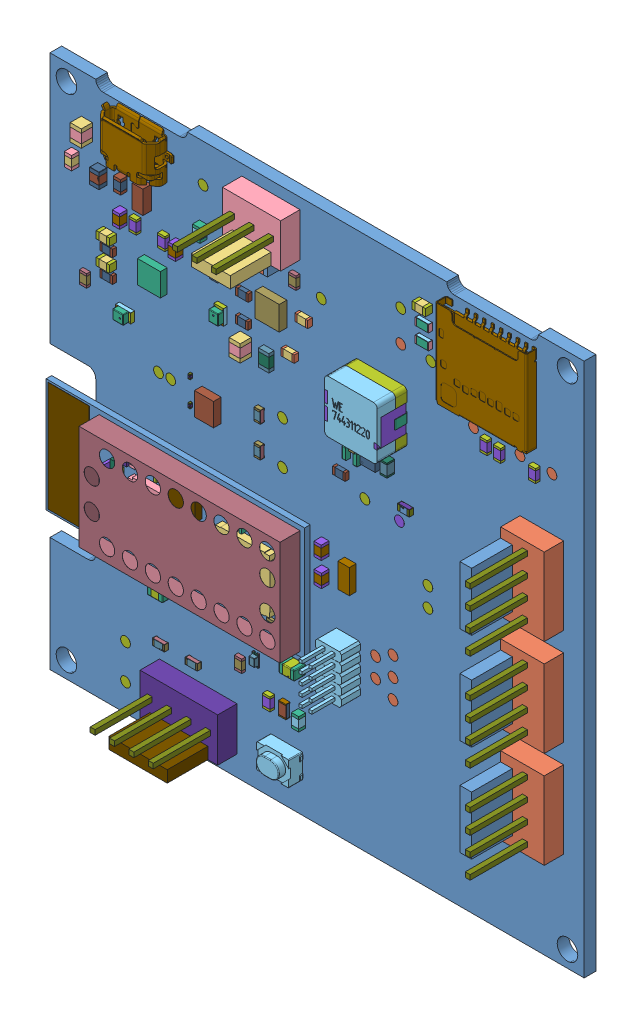
SolidWorks assembly IoTracking_PCB_new, configuration Default. Lengths in mm. (continued)
Components (placement in the parent): (continued)
- IoTracking_PCB_new.step-1: IoTracking_PCB_new.step [Default] at origin size (70.02 70.02 13.59) (continued)
  - R11.step-1: R11.step [Default] at origin size (0.95 1.65 0.5) (continued)
    - 6125954368.step-1: 6125954368.step [Default] at (25.146 13.4112 0) size (0.95 1.05 0.5)
      - Extruded-18.step-1: Extruded-18.step [Default] at origin size (0.95 1.05 0.5)
    - 6125954208.step-1: 6125954208.step [Default] at (25.146 12.7362 0) size (0.95 0.3 0.5)
      - Extruded-19.step-1: Extruded-19.step [Default] at origin size (0.95 0.3 0.5)
    - 6125954208.step-2: 6125954208.step [Default] at (25.146 14.0862 0) size (0.95 0.3 0.5)
      - Extruded-19.step-1: Extruded-19.step [Default] at origin size (0.95 0.3 0.5)
  - R10.step-1: R10.step [Default] at origin size (0.95 1.7 0.6)
    - 6127426432.step-1: 6127426432.step [Default] at (59.1819 55.0711 0) size (0.95 0.27 0.6)
      - Extruded-13.step-1: Extruded-13.step [Default] at origin size (0.95 0.27 0.6)
    - 6127426272.step-1: 6127426272.step [Default] at (59.1819 54.3561 0) size (0.95 1.16 0.6)
      - Extruded-14.step-1: Extruded-14.step [Default] at origin size (0.95 1.16 0.6)
    - 6127426432.step-2: 6127426432.step [Default] at (59.1819 53.6411 0) size (0.95 0.27 0.6)
      - Extruded-13.step-1: Extruded-13.step [Default] at origin size (0.95 0.27 0.6)
  - R9.step-1: R9.step [Default] at origin size (0.95 1.7 0.6)
    - 6127426432.step-1: 6127426432.step [Default] at (63.7539 55.0711 0) size (0.95 0.27 0.6)
      - Extruded-13.step-1: Extruded-13.step [Default] at origin size (0.95 0.27 0.6)
    - 6127426272.step-1: 6127426272.step [Default] at (63.7539 54.3561 0) size (0.95 1.16 0.6)
      - Extruded-14.step-1: Extruded-14.step [Default] at origin size (0.95 1.16 0.6)
    - 6127426432.step-2: 6127426432.step [Default] at (63.7539 53.6411 0) size (0.95 0.27 0.6)
      - Extruded-13.step-1: Extruded-13.step [Default] at origin size (0.95 0.27 0.6)
  - R8.step-1: R8.step [Default] at origin size (0.95 1.7 0.6)
    - 6127426432.step-1: 6127426432.step [Default] at (57.4039 55.0711 0) size (0.95 0.27 0.6)
      - Extruded-13.step-1: Extruded-13.step [Default] at origin size (0.95 0.27 0.6)
    - 6127426272.step-1: 6127426272.step [Default] at (57.4039 54.3561 0) size (0.95 1.16 0.6)
      - Extruded-14.step-1: Extruded-14.step [Default] at origin size (0.95 1.16 0.6)
    - 6127426432.step-2: 6127426432.step [Default] at (57.4039 53.6411 0) size (0.95 0.27 0.6)
      - Extruded-13.step-1: Extruded-13.step [Default] at origin size (0.95 0.27 0.6)
  - R7.step-1: R7.step [Default] at origin size (0.95 1.65 0.5)
    - 6125954208.step-1: 6125954208.step [Default] at (32.258 61.127 0) size (0.95 0.3 0.5)
      - Extruded-19.step-1: Extruded-19.step [Default] at origin size (0.95 0.3 0.5)
    - 6125954208.step-2: 6125954208.step [Default] at (32.258 59.777 0) size (0.95 0.3 0.5)
      - Extruded-19.step-1: Extruded-19.step [Default] at origin size (0.95 0.3 0.5)
    - 6125954368.step-1: 6125954368.step [Default] at (32.258 60.452 0) size (0.95 1.05 0.5)
      - Extruded-18.step-1: Extruded-18.step [Default] at origin size (0.95 1.05 0.5)
  - R6.step-1: R6.step [Default] at origin size (1.35 2.2 0.7)
    - 6127414912.step-1: 6127414912.step [Default] at (28.7021 48.8939 0) size (1.35 0.42 0.7)
      - Extruded-20.step-1: Extruded-20.step [Default] at origin size (1.35 0.42 0.7)
    - 6127414752.step-1: 6127414752.step [Default] at (28.7021 49.7839 0) size (1.35 1.36 0.7)
      - Extruded-21.step-1: Extruded-21.step [Default] at origin size (1.35 1.36 0.7)
    - 6127414912.step-2: 6127414912.step [Default] at (28.7021 50.6739 0) size (1.35 0.42 0.7)
      - Extruded-20.step-1: Extruded-20.step [Default] at origin size (1.35 0.42 0.7)
  - R5.step-1: R5.step [Default] at origin size (1.65 0.95 0.5)
    - 6125952048.step-1: 6125952048.step [Default] at (7.874 48.768 0) size (1.05 0.95 0.5)
      - Extruded-7.step-1: Extruded-7.step [Default] at origin size (1.05 0.95 0.5)
    - 6125951888.step-1: 6125951888.step [Default] at (7.199 48.768 0) size (0.3 0.95 0.5)
      - Extruded-8.step-1: Extruded-8.step [Default] at origin size (0.3 0.95 0.5)
    - 6125951888.step-2: 6125951888.step [Default] at (8.549 48.768 0) size (0.3 0.95 0.5)
      - Extruded-8.step-1: Extruded-8.step [Default] at origin size (0.3 0.95 0.5)
  - R4.step-1: R4.step [Default] at origin size (1.65 0.95 0.5)
    - 6125951888.step-1: 6125951888.step [Default] at (8.549 51.816 0) size (0.3 0.95 0.5)
      - Extruded-8.step-1: Extruded-8.step [Default] at origin size (0.3 0.95 0.5)
    - 6125951888.step-2: 6125951888.step [Default] at (7.199 51.816 0) size (0.3 0.95 0.5)
      - Extruded-8.step-1: Extruded-8.step [Default] at origin size (0.3 0.95 0.5)
    - 6125952048.step-1: 6125952048.step [Default] at (7.874 51.816 0) size (1.05 0.95 0.5)
      - Extruded-7.step-1: Extruded-7.step [Default] at origin size (1.05 0.95 0.5)
  - R3.step-1: R3.step [Default] at origin size (0.95 1.65 0.5)
    - 6125954208.step-1: 6125954208.step [Default] at (4.826 47.665 0) size (0.95 0.3 0.5)
      - Extruded-19.step-1: Extruded-19.step [Default] at origin size (0.95 0.3 0.5)
    - 6125954208.step-2: 6125954208.step [Default] at (4.826 46.315 0) size (0.95 0.3 0.5)
      - Extruded-19.step-1: Extruded-19.step [Default] at origin size (0.95 0.3 0.5)
    - 6125954368.step-1: 6125954368.step [Default] at (4.826 46.99 0) size (0.95 1.05 0.5)
      - Extruded-18.step-1: Extruded-18.step [Default] at origin size (0.95 1.05 0.5)
  - R2.step-1: R2.step [Default] at origin size (0.95 1.7 0.6)
    - 6127426432.step-1: 6127426432.step [Default] at (15.1893 55.6857 0) size (0.95 0.27 0.6)
      - Extruded-13.step-1: Extruded-13.step [Default] at origin size (0.95 0.27 0.6)
    - 6127426272.step-1: 6127426272.step [Default] at (15.1893 56.4007 0) size (0.95 1.16 0.6)
      - Extruded-14.step-1: Extruded-14.step [Default] at origin size (0.95 1.16 0.6)
    - 6127426432.step-2: 6127426432.step [Default] at (15.1893 57.1157 0) size (0.95 0.27 0.6)
      - Extruded-13.step-1: Extruded-13.step [Default] at origin size (0.95 0.27 0.6)
  - R1.step-1: R1.step [Default] at origin size (0.95 1.7 0.6)
    - 6127426432.step-1: 6127426432.step [Default] at (11.4301 55.6729 0) size (0.95 0.27 0.6)
      - Extruded-13.step-1: Extruded-13.step [Default] at origin size (0.95 0.27 0.6)
    - 6127426272.step-1: 6127426272.step [Default] at (11.4301 56.3879 0) size (0.95 1.16 0.6)
      - Extruded-14.step-1: Extruded-14.step [Default] at origin size (0.95 1.16 0.6)
    - 6127426432.step-2: 6127426432.step [Default] at (11.4301 57.1029 0) size (0.95 0.27 0.6)
      - Extruded-13.step-1: Extruded-13.step [Default] at origin size (0.95 0.27 0.6)
  - P5.step-1: P5.step [Default] at origin size (10.16 5.72 13.59)
    - 6127411952.step-1: 6127411952.step [Default] at (20.7009 5.8419 -3.56) size (0.64 0.64 13.59)
      - Extruded-22.step-1: Extruded-22.step [Default] at origin size (0.64 0.64 13.59)
    - 6127411952.step-2: 6127411952.step [Default] at (18.1609 5.842 -3.56) size (0.64 0.64 13.59)
      - Extruded-22.step-1: Extruded-22.step [Default] at origin size (0.64 0.64 13.59)
    - 6127411952.step-3: 6127411952.step [Default] at (15.6209 5.8418 -3.56) size (0.64 0.64 13.59)
      - Extruded-22.step-1: Extruded-22.step [Default] at origin size (0.64 0.64 13.59)
    - 6127411952.step-4: 6127411952.step [Default] at (23.2409 5.8419 -3.56) size (0.64 0.64 13.59)
      - Extruded-22.step-1: Extruded-22.step [Default] at origin size (0.64 0.64 13.59)
    - 6125956208.step-1: 6125956208.step [Default] at (19.431 5.5245 0) size (10.16 5.71 2.54)
      - Extruded-23.step-1: Extruded-23.step [Default] at origin size (10.16 5.71 2.54)
    - 6125956048.step-1: 6125956048.step [Default] at (19.431 3.4265 2.54) size (7.62 1.53 5.33)
      - Extruded-24.step-1: Extruded-24.step [Default] at origin size (7.62 1.53 5.33)
  - P4.step-1: P4.step [Default] at origin size (5.72 10.16 13.59)
    - 6125954528.step-1: 6125954528.step [Default] at (62.3545 17.78 2.54) size (1.53 7.62 5.33)
      - Extruded-25.step-1: Extruded-25.step [Default] at origin size (1.53 7.62 5.33)
    - 6125954688.step-1: 6125954688.step [Default] at (64.4525 17.78 0) size (5.71 10.16 2.54)
      - Extruded-26.step-1: Extruded-26.step [Default] at origin size (5.71 10.16 2.54)
    - 6127411952.step-1: 6127411952.step [Default] at (64.7699 13.9701 -3.56) size (0.64 0.64 13.59)
      - Extruded-22.step-1: Extruded-22.step [Default] at origin size (0.64 0.64 13.59)
    - 6127411952.step-2: 6127411952.step [Default] at (64.7698 21.5901 -3.56) size (0.64 0.64 13.59)
      - Extruded-22.step-1: Extruded-22.step [Default] at origin size (0.64 0.64 13.59)
    - 6127411952.step-3: 6127411952.step [Default] at (64.7699 19.0501 -3.56) size (0.64 0.64 13.59)
      - Extruded-22.step-1: Extruded-22.step [Default] at origin size (0.64 0.64 13.59)
    - 6127411952.step-4: 6127411952.step [Default] at (64.7699 16.5101 -3.56) size (0.64 0.64 13.59)
      - Extruded-22.step-1: Extruded-22.step [Default] at origin size (0.64 0.64 13.59)
  - P3.step-1: P3.step [Default] at origin size (5.72 10.16 13.59)
    - 6127411952.step-1: 6127411952.step [Default] at (64.7699 29.2101 -3.56) size (0.64 0.64 13.59)
      - Extruded-22.step-1: Extruded-22.step [Default] at origin size (0.64 0.64 13.59)
    - 6127411952.step-2: 6127411952.step [Default] at (64.7699 31.7501 -3.56) size (0.64 0.64 13.59)
      - Extruded-22.step-1: Extruded-22.step [Default] at origin size (0.64 0.64 13.59)
    - 6127411952.step-3: 6127411952.step [Default] at (64.7698 34.2901 -3.56) size (0.64 0.64 13.59)
      - Extruded-22.step-1: Extruded-22.step [Default] at origin size (0.64 0.64 13.59)
    - 6127411952.step-4: 6127411952.step [Default] at (64.7699 26.6701 -3.56) size (0.64 0.64 13.59)
      - Extruded-22.step-1: Extruded-22.step [Default] at origin size (0.64 0.64 13.59)
    - 6125954688.step-1: 6125954688.step [Default] at (64.4525 30.48 0) size (5.71 10.16 2.54)
      - Extruded-26.step-1: Extruded-26.step [Default] at origin size (5.71 10.16 2.54)
    - 6125954528.step-1: 6125954528.step [Default] at (62.3545 30.48 2.54) size (1.53 7.62 5.33)
      - Extruded-25.step-1: Extruded-25.step [Default] at origin size (1.53 7.62 5.33)
  - P2.step-1: P2.step [Default] at origin size (5.72 10.16 13.59)
    - 6125954528.step-1: 6125954528.step [Default] at (62.3545 43.18 2.54) size (1.53 7.62 5.33)
      - Extruded-25.step-1: Extruded-25.step [Default] at origin size (1.53 7.62 5.33)
    - 6125954688.step-1: 6125954688.step [Default] at (64.4525 43.18 0) size (5.71 10.16 2.54)
      - Extruded-26.step-1: Extruded-26.step [Default] at origin size (5.71 10.16 2.54)
    - 6127411952.step-1: 6127411952.step [Default] at (64.7699 39.3701 -3.56) size (0.64 0.64 13.59)
      - Extruded-22.step-1: Extruded-22.step [Default] at origin size (0.64 0.64 13.59)
    - 6127411952.step-2: 6127411952.step [Default] at (64.7698 46.9901 -3.56) size (0.64 0.64 13.59)
      - Extruded-22.step-1: Extruded-22.step [Default] at origin size (0.64 0.64 13.59)
    - 6127411952.step-3: 6127411952.step [Default] at (64.7699 44.4501 -3.56) size (0.64 0.64 13.59)
      - Extruded-22.step-1: Extruded-22.step [Default] at origin size (0.64 0.64 13.59)
    - 6127411952.step-4: 6127411952.step [Default] at (64.7699 41.9101 -3.56) size (0.64 0.64 13.59)
      - Extruded-22.step-1: Extruded-22.step [Default] at origin size (0.64 0.64 13.59)
  - P1.step-1: P1.step [Default] at origin size (7.62 5.72 13.59)
    - 6127411472.step-1: 6127411472.step [Default] at (28.956 63.627 2.54) size (5.08 1.52 5.33)
      - Extruded-27.step-1: Extruded-27.step [Default] at origin size (5.08 1.52 5.33)
    - 6127411632.step-1: 6127411632.step [Default] at (28.956 65.7225 0) size (7.62 5.71 2.54)
      - Extruded-28.step-1: Extruded-28.step [Default] at origin size (7.62 5.71 2.54)
    - 6127411952.step-1: 6127411952.step [Default] at (31.4959 66.0399 -3.56) size (0.64 0.64 13.59)
      - Extruded-22.step-1: Extruded-22.step [Default] at origin size (0.64 0.64 13.59)
    - 6127411952.step-2: 6127411952.step [Default] at (26.4159 66.0399 -3.56) size (0.64 0.64 13.59)
      - Extruded-22.step-1: Extruded-22.step [Default] at origin size (0.64 0.64 13.59)
    - 6127411952.step-3: 6127411952.step [Default] at (28.9559 66.0399 -3.56) size (0.64 0.64 13.59)
      - Extruded-22.step-1: Extruded-22.step [Default] at origin size (0.64 0.64 13.59)
  - L_B1.step-1: L_B1.step [Default] at origin size (7.01 6.9 4)
    - 744311220.step-1: 744311220.step [Default] at (43.434 52.07 1.6) x (0 1 0) z (0 0 1) size (6.9 7.01 4)
      - Geh_use.step-1: Geh_use.step [Default] at origin size (6.9 6.9 2.4)
      - Spule.step-1: Spule.step [Default] at (0 0 -0.0088) x (0 -1 0) z (0 0 1) size (7.01 5.89 3.39)
      - Boden.step-1: Boden.step [Default] at (0 0 -1.5) size (6.9 6.9 1.5)
      - Klebemasse.step-1: Klebemasse.step [Default] at (0 3.25 0) x (-1 0 0) z (0 0 1) size (3.5 0.4 3.8)
      - Klebemasse.step-2: Klebemasse.step [Default] at (0 -3.25 0) size (3.5 0.4 3.8)
  - J1.step-1: J1.step [Default] at origin size (8.8 5.73 2.94)
    - ZX62R-B-5P.step-1: ZX62R-B-5P.step [Default] at (13.238 63.2505 0) x (-1 0 0) z (0 1 0) size (8.8 2.94 5.73)
  - FB1.step-1: FB1.step [Default] at origin size (1.25 2 1.05)
    - FBead_Murata_BLM21AG102SN1D_eec.step-1: FBead_Murata_BLM21AG102SN1D_eec.step [Default] at (6.858 59.69 0) x (0 1 0) z (0 0 1) size (2 1.25 1.05)
      - Electrodes.step-1: Electrodes.step [Default] at origin size (2 1.25 1.05)
      - Dielectric.step-1: Dielectric.step [Default] at origin size (1 1.24 1.04)
      - Murata.step-1: Murata.step [Default] at origin size (0.53 0.12 0)
  - DS1.step-1: DS1.step [Default] at origin size (0.8 1.6 0.65)
    - Diode_Lite-On_LTST-C191KGKT_eec.step-1: Diode_Lite-On_LTST-C191KGKT_eec.step [Default] at (27.0764 14.732 0) x (0 -1 0) z (0 0 1) size (1.6 0.8 0.65)
      - 1-29.step-1: 1-29.step [Default] at origin size (1.6 0.8 0.16)
      - 2-30.step-1: 2-30.step [Default] at origin size (1.1 0.8 0.47)
      - 3-31.step-1: 3-31.step [Default] at origin size (1.6 0.7 0.18)
      - Lite-On_Logo_Adjustable.step-1: Lite-On_Logo_Adjustable.step [Default] at (-0.9403 -0.3001 -1.9063) x (1 0 0) z (0 -1 0) size (0.21 0.05 0.1)
  - D4.step-1: D4.step [Default] at origin size (1.25 2 1.2)
    - Diode_Lite-On_LTST-C170GKT_eec.step-1: Diode_Lite-On_LTST-C170GKT_eec.step [Default] at (22.606 56.642 0) x (1 0 0) z (0 0 1) size (1.25 2 1.2)
      - 1-32.step-1: 1-32.step [Default] at origin size (0.15 0.15 0.05)
      - 2-33.step-1: 2-33.step [Default] at origin size (1.25 2 0.5)
      - 3-34.step-1: 3-34.step [Default] at origin size (1.25 1.4 0.75)
      - 4-35.step-1: 4-35.step [Default] at origin size (1.25 1.9 0.4)
      - Lite-On_Logo_Adjustable-36.step-1: Lite-On_Logo_Adjustable-36.step [Default] at (0.526 -1.0018 -1.9007) x (0 1 0) z (1 0 0) size (0.43 0.1 0.1)
      - 5-37.step-1: 5-37.step [Default] at origin size (1.25 0.3 0.03)
  - D3.step-1: D3.step [Default] at origin size (1.25 2 1.2)
    - Diode_Lite-On_LTST-C170CKT_eec.step-1: Diode_Lite-On_LTST-C170CKT_eec.step [Default] at (22.606 51.816 0) x (0 -1 0) z (0 0 1) size (2 1.25 1.2)
      - pcb.step-1: pcb.step [Default] at (0 0 0.01) size (1.98 1.25 0.48)
      - top.step-1: top.step [Default] at (0 0 0.49) size (1.4 1.25 0.71)
      - lead.step-1: lead.step [Default] at (-0.7501 0 0.5) x (-1 0 0) z (0 0 -1) size (0.5 1.25 0.5)
      - emitter.step-1: emitter.step [Default] at (-0.0551 -0.005 1.2) size (0.15 0.15 0)
      - lead_MIR1.step-1: lead_MIR1.step [Default] at (0.7499 0 0.5) size (0.5 1.25 0.5)
      - marking.step-1: marking.step [Default] at (-0.9399 0 0.5) size (0.31 1.25 0)
  - D2.step-1: D2.step [Default] at origin size (1.4 3 1.1)
    - 6127411312.step-1: 6127411312.step [Default] at (12.573 60.198 0) size (1.4 3 1.1)
      - Extruded-38.step-1: Extruded-38.step [Default] at origin size (1.4 3 1.1)
  - D1.step-1: D1.step [Default] at origin size (2 1.25 1.2)
    - Diode_Lite-On_LTST-C170CKT_eec.step-1: Diode_Lite-On_LTST-C170CKT_eec.step [Default] at (10.086 45.6292 0) x (-1 0 0) z (0 0 1) size (2 1.25 1.2)
      - pcb.step-1: pcb.step [Default] at (0 0 0.01) size (1.98 1.25 0.48)
      - top.step-1: top.step [Default] at (0 0 0.49) size (1.4 1.25 0.71)
      - lead.step-1: lead.step [Default] at (-0.7501 0 0.5) x (-1 0 0) z (0 0 -1) size (0.5 1.25 0.5)
      - emitter.step-1: emitter.step [Default] at (-0.0551 -0.005 1.2) size (0.15 0.15 0)
      - lead_MIR1.step-1: lead_MIR1.step [Default] at (0.7499 0 0.5) size (0.5 1.25 0.5)
      - marking.step-1: marking.step [Default] at (-0.9399 0 0.5) size (0.31 1.25 0)
  - C_B2.step-1: C_B2.step [Default] at origin size (2.01 2.72 1.43)
    - Cap_TDK_Corporation_C1608X5R1C106M080AB_eec.step-1: Cap_TDK_Corporation_C1608X5R1C106M080AB_eec.step [Default] at (40.259 45.782 0) x (0 -1 0) z (0 0 1) size (2.72 2.01 1.43)
      - body.step-1: body.step [Default] at origin size (1.2 0.8 0.8)
      - Terminals.step-1: Terminals.step [Default] at (0.6 -0.4 0) x (0 1 0) z (1 0 0) size (2.01 1.25 1.52)
      - value.step-1: value.step [Default] at (0 0 0.8) size (0.79 0.68 0.25)
  - C_B1.step-1: C_B1.step [Default] at origin size (0.9 1.7 1)
    - 6125950048.step-1: 6125950048.step [Default] at (44.704 45.632 0) size (0.9 1.3 1)
      - Extruded-39.step-1: Extruded-39.step [Default] at origin size (0.9 1.3 1)
    - 6125949888.step-1: 6125949888.step [Default] at (44.704 44.882 0) size (0.9 0.2 1)
      - Extruded-40.step-1: Extruded-40.step [Default] at origin size (0.9 0.2 1)
    - 6125949888.step-2: 6125949888.step [Default] at (44.704 46.382 0) size (0.9 0.2 1)
      - Extruded-40.step-1: Extruded-40.step [Default] at origin size (0.9 0.2 1)
  - C_A2.step-1: C_A2.step [Default] at origin size (0.3 0.6 0.34)
    - Cap_Murata_GRM0335C1HR30BA01D_eec.step-1: Cap_Murata_GRM0335C1HR30BA01D_eec.step [Default] at (18.542 39.37 0) x (0 1 0) z (0 0 1) size (0.6 0.3 0.34)
      - terminals-41.step-1: terminals-41.step [Default] at origin size (0.6 0.3 0.33)
      - body-42.step-1: body-42.step [Default] at origin size (0.3 0.3 0.33)
      - logo.step-1: logo.step [Default] at (-0.2332 0.5956 0.33) size (0.25 0.06 0.01)
  - C_A1.step-1: C_A1.step [Default] at origin size (0.3 0.6 0.34)
    - Cap_Murata_GRM0335C1HR30BA01D_eec.step-1: Cap_Murata_GRM0335C1HR30BA01D_eec.step [Default] at (18.542 42.672 0) x (0 1 0) z (0 0 1) size (0.6 0.3 0.34)
      - terminals-41.step-1: terminals-41.step [Default] at origin size (0.6 0.3 0.33)
      - body-42.step-1: body-42.step [Default] at origin size (0.3 0.3 0.33)
      - logo.step-1: logo.step [Default] at (-0.2332 0.5956 0.33) size (0.25 0.06 0.01)
  - C16.step-1: C16.step [Default] at origin size (2.2 1.45 1.45)
    - 6127425232.step-1: 6127425232.step [Default] at (27.99 60.96 0) size (0.5 1.45 1.45)
      - Extruded-43.step-1: Extruded-43.step [Default] at origin size (0.5 1.45 1.45)
    - 6127425232.step-2: 6127425232.step [Default] at (29.69 60.96 0) size (0.5 1.45 1.45)
      - Extruded-43.step-1: Extruded-43.step [Default] at origin size (0.5 1.45 1.45)
    - 6127425392.step-1: 6127425392.step [Default] at (28.84 60.96 0) size (1.2 1.45 1.45)
      - Extruded-44.step-1: Extruded-44.step [Default] at origin size (1.2 1.45 1.45)
  - C15.step-1: C15.step [Default] at origin size (1.45 2.2 1.45)
    - 6125947888.step-1: 6125947888.step [Default] at (25.654 50.634 0) size (1.45 0.5 1.45)
      - Extruded-45.step-1: Extruded-45.step [Default] at origin size (1.45 0.5 1.45)
    - 6125947888.step-2: 6125947888.step [Default] at (25.654 48.934 0) size (1.45 0.5 1.45)
      - Extruded-45.step-1: Extruded-45.step [Default] at origin size (1.45 0.5 1.45)
    - 6125947648.step-1: 6125947648.step [Default] at (25.654 49.784 0) size (1.45 1.2 1.45)
      - Extruded-46.step-1: Extruded-46.step [Default] at origin size (1.45 1.2 1.45)
  - C14.step-1: C14.step [Default] at origin size (0.96 1.75 0.9)
    - 6125952448.step-1: 6125952448.step [Default] at (20.066 59.944 0) size (0.96 1.05 0.9)
      - Extruded-47.step-1: Extruded-47.step [Default] at origin size (0.96 1.05 0.9)
    - 6125952288.step-1: 6125952288.step [Default] at (20.066 59.244 0) size (0.96 0.35 0.9)
      - Extruded-48.step-1: Extruded-48.step [Default] at origin size (0.96 0.35 0.9)
    - 6125952288.step-2: 6125952288.step [Default] at (20.066 60.644 0) size (0.96 0.35 0.9)
      - Extruded-48.step-1: Extruded-48.step [Default] at origin size (0.96 0.35 0.9)
  - C13.step-1: C13.step [Default] at origin size (1.75 0.95 0.95)
    - 6125953728.step-1: 6125953728.step [Default] at (49.276 66.04 0) size (0.95 0.95 0.95)
      - Extruded.step-1: Extruded.step [Default] at origin size (0.95 0.95 0.95)
    - 6125949568.step-1: 6125949568.step [Default] at (49.951 66.04 0) size (0.4 0.95 0.95)
      - Extruded-49.step-1: Extruded-49.step [Default] at origin size (0.4 0.95 0.95)
    - 6125949568.step-2: 6125949568.step [Default] at (48.601 66.04 0) size (0.4 0.95 0.95)
      - Extruded-49.step-1: Extruded-49.step [Default] at origin size (0.4 0.95 0.95)
  - C12.step-1: C12.step [Default] at origin size (0.95 1.75 1)
    - 6127425632.step-1: 6127425632.step [Default] at (36.068 31.304 0) size (0.95 0.35 1)
      - Extruded-50.step-1: Extruded-50.step [Default] at origin size (0.95 0.35 1)
    - 6127425632.step-2: 6127425632.step [Default] at (36.068 32.704 0) size (0.95 0.35 1)
      - Extruded-50.step-1: Extruded-50.step [Default] at origin size (0.95 0.35 1)
    - 6127425792.step-1: 6127425792.step [Default] at (36.068 32.004 0) size (0.95 1.05 1)
      - Extruded-51.step-1: Extruded-51.step [Default] at origin size (0.95 1.05 1)
  - C11.step-1: C11.step [Default] at origin size (0.95 1.75 1)
    - 6127425632.step-1: 6127425632.step [Default] at (36.0934 29.529 0) size (0.95 0.35 1)
      - Extruded-50.step-1: Extruded-50.step [Default] at origin size (0.95 0.35 1)
    - 6127425632.step-2: 6127425632.step [Default] at (36.0934 28.129 0) size (0.95 0.35 1)
      - Extruded-50.step-1: Extruded-50.step [Default] at origin size (0.95 0.35 1)
    - 6127425792.step-1: 6127425792.step [Default] at (36.0934 28.829 0) size (0.95 1.05 1)
      - Extruded-51.step-1: Extruded-51.step [Default] at origin size (0.95 1.05 1)
  - C10.step-1: C10.step [Default] at origin size (0.96 1.75 0.9)
    - 6125952448.step-1: 6125952448.step [Default] at (33.02 10.9728 0) size (0.96 1.05 0.9)
      - Extruded-47.step-1: Extruded-47.step [Default] at origin size (0.96 1.05 0.9)
    - 6125952288.step-1: 6125952288.step [Default] at (33.02 10.2728 0) size (0.96 0.35 0.9)
      - Extruded-48.step-1: Extruded-48.step [Default] at origin size (0.96 0.35 0.9)
    - 6125952288.step-2: 6125952288.step [Default] at (33.02 11.6728 0) size (0.96 0.35 0.9)
      - Extruded-48.step-1: Extruded-48.step [Default] at origin size (0.96 0.35 0.9)
  - C8.step-1: C8.step [Default] at origin size (2.01 1.25 1.52)
    - Cap_AVX_0805YA103FAT2A_eec.step-1: Cap_AVX_0805YA103FAT2A_eec.step [Default] at (15.24 17.018 0) x (-1 0 0) z (0 0 1) size (2.01 1.25 1.52)
      - Terminals.step-1: Terminals.step [Default] at origin size (2.01 1.25 1.52)
      - Electrode.step-1: Electrode.step [Default] at origin size (1.01 1.25 1.52)
      - AVX.step-1: AVX.step [Default] at origin size (0.37 0.13 0)
  - C7.step-1: C7.step [Default] at origin size (1.75 0.95 0.95)
    - 6125953728.step-1: 6125953728.step [Default] at (7.874 50.292 0) size (0.95 0.95 0.95)
      - Extruded.step-1: Extruded.step [Default] at origin size (0.95 0.95 0.95)
    - 6125949568.step-1: 6125949568.step [Default] at (7.199 50.292 0) size (0.4 0.95 0.95)
      - Extruded-49.step-1: Extruded-49.step [Default] at origin size (0.4 0.95 0.95)
    - 6125949568.step-2: 6125949568.step [Default] at (8.549 50.292 0) size (0.4 0.95 0.95)
      - Extruded-49.step-1: Extruded-49.step [Default] at origin size (0.4 0.95 0.95)
  - C6.step-1: C6.step [Default] at origin size (0.95 1.75 1)
    - 6127425632.step-1: 6127425632.step [Default] at (16.9672 57.1008 0) size (0.95 0.35 1)
      - Extruded-50.step-1: Extruded-50.step [Default] at origin size (0.95 0.35 1)
    - 6127425632.step-2: 6127425632.step [Default] at (16.9672 55.7008 0) size (0.95 0.35 1)
      - Extruded-50.step-1: Extruded-50.step [Default] at origin size (0.95 0.35 1)
    - 6127425792.step-1: 6127425792.step [Default] at (16.9672 56.4008 0) size (0.95 1.05 1)
      - Extruded-51.step-1: Extruded-51.step [Default] at origin size (0.95 1.05 1)
  - C5.step-1: C5.step [Default] at origin size (0.95 1.75 1)
    - 6127425632.step-1: 6127425632.step [Default] at (9.652 57.088 0) size (0.95 0.35 1)
      - Extruded-50.step-1: Extruded-50.step [Default] at origin size (0.95 0.35 1)
    - 6127425632.step-2: 6127425632.step [Default] at (9.652 55.688 0) size (0.95 0.35 1)
      - Extruded-50.step-1: Extruded-50.step [Default] at origin size (0.95 0.35 1)
    - 6127425792.step-1: 6127425792.step [Default] at (9.652 56.388 0) size (0.95 1.05 1)
      - Extruded-51.step-1: Extruded-51.step [Default] at origin size (0.95 1.05 1)
  - C4.step-1: C4.step [Default] at origin size (1.45 2.2 1.45)
    - 6125947888.step-1: 6125947888.step [Default] at (4.826 62.904 0) size (1.45 0.5 1.45)
      - Extruded-45.step-1: Extruded-45.step [Default] at origin size (1.45 0.5 1.45)
    - 6125947888.step-2: 6125947888.step [Default] at (4.826 64.604 0) size (1.45 0.5 1.45)
      - Extruded-45.step-1: Extruded-45.step [Default] at origin size (1.45 0.5 1.45)
    - 6125947648.step-1: 6125947648.step [Default] at (4.826 63.754 0) size (1.45 1.2 1.45)
      - Extruded-46.step-1: Extruded-46.step [Default] at origin size (1.45 1.2 1.45)
  - C2.step-1: C2.step [Default] at origin size (0.95 1.75 0.87)
    - 6125945248.step-1: 6125945248.step [Default] at (9.652 60.198 0) size (0.95 1.05 0.87)
      - Extruded-52.step-1: Extruded-52.step [Default] at origin size (0.95 1.05 0.87)
    - 6125945088.step-1: 6125945088.step [Default] at (9.652 60.898 0) size (0.95 0.35 0.87)
      - Extruded-53.step-1: Extruded-53.step [Default] at origin size (0.95 0.35 0.87)
    - 6125945088.step-2: 6125945088.step [Default] at (9.652 59.498 0) size (0.95 0.35 0.87)
      - Extruded-53.step-1: Extruded-53.step [Default] at origin size (0.95 0.35 0.87)
  - C1.step-1: C1.step [Default] at origin size (1.75 0.95 0.95)
    - 6125953728.step-1: 6125953728.step [Default] at (7.874 53.34 0) size (0.95 0.95 0.95)
      - Extruded.step-1: Extruded.step [Default] at origin size (0.95 0.95 0.95)
    - 6125949568.step-1: 6125949568.step [Default] at (7.199 53.34 0) size (0.4 0.95 0.95)
      - Extruded-49.step-1: Extruded-49.step [Default] at origin size (0.4 0.95 0.95)
    - 6125949568.step-2: 6125949568.step [Default] at (8.549 53.34 0) size (0.4 0.95 0.95)
      - Extruded-49.step-1: Extruded-49.step [Default] at origin size (0.4 0.95 0.95)
  - Free-Models.step-1: Free-Models.step [Default] at origin size (70 70 10)
    - boardSmall.step-1: boardSmall.step [Default] at (34.977 34.9758 0) size (70 70 10) (hidden)
